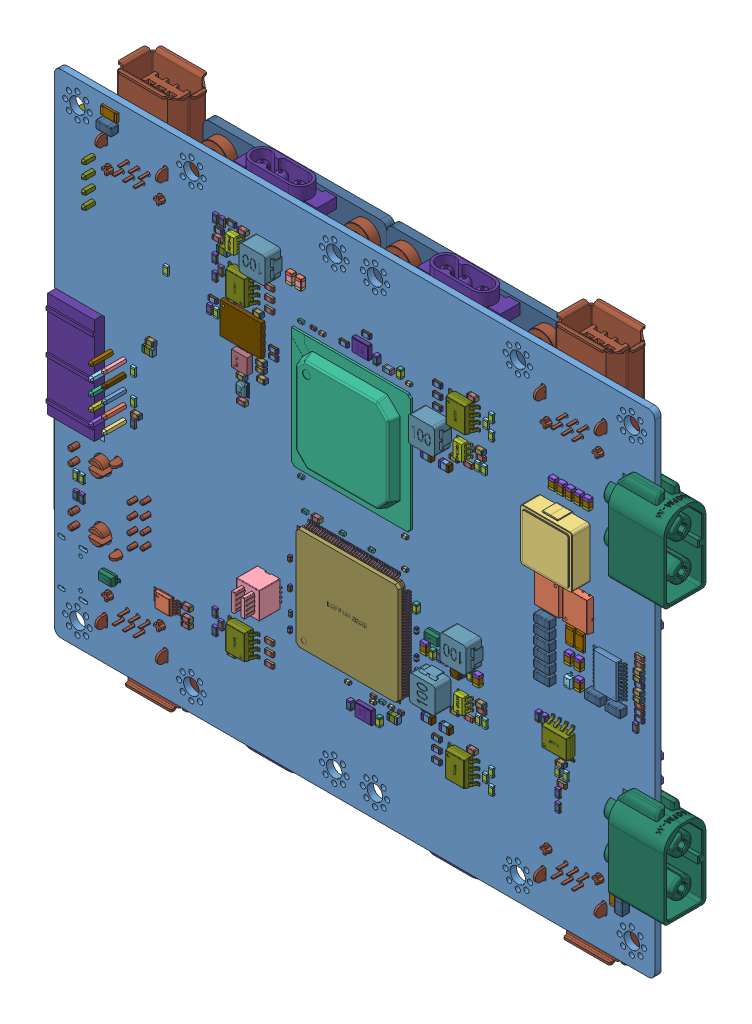
SolidWorks assembly Mother  Board, configuration 默认. Lengths in mm. (continued)
Components (placement in the parent): (continued)
- Mother  Board.step-1: Mother  Board.step [默认] at origin size (122.6 102.08 21) (continued)
  - R4_D2.step-1: R4_D2.step [默认] at origin size (0.8 1.6 0.45) (continued)
    - 5993842864.step-1: 5993842864.step [默认] at (78.9939 13.4621 0) x (0 1 0) z (0 0 1) size (1.6 0.8 0.45) (continued)
      - Terminal-12.step-1: Terminal-12.step [默认] at (-0.8 -0.4 0) size (0.3 0.8 0.45)
        - Open_CASCADE_STEP_translator_6.8_21.2.1-28.step-1: Open_CASCADE_STEP_translator_6.8_21.2.1-28.step [默认] at origin size (0.3 0.8 0.45)
      - Terminal-12.step-2: Terminal-12.step [默认] at (0.8 0.4 0) x (-1 0 0) z (0 0 1) size (0.3 0.8 0.45)
        - Open_CASCADE_STEP_translator_6.8_21.2.1-28.step-1: Open_CASCADE_STEP_translator_6.8_21.2.1-28.step [默认] at origin size (0.3 0.8 0.45)
      - Mid_Body-29.step-1: Mid_Body-29.step [默认] at (-0.8 -0.4 0) size (1.51 0.8 0.36)
      - Mark-30.step-1: Mark-30.step [默认] at (-0.5 -0.4 0.405) size (1 0.8 0.05)
  - R4_D1.step-1: R4_D1.step [默认] at origin size (0.8 1.6 0.45)
    - 5993843024.step-1: 5993843024.step [默认] at (27.9401 13.4619 0) x (0 -1 0) z (0 0 1) size (1.6 0.8 0.45)
      - Terminal-13.step-1: Terminal-13.step [默认] at (-0.8 -0.4 0) size (0.3 0.8 0.45)
        - Open_CASCADE_STEP_translator_6.8_21.2.1-31.step-1: Open_CASCADE_STEP_translator_6.8_21.2.1-31.step [默认] at origin size (0.3 0.8 0.45)
      - Terminal-13.step-2: Terminal-13.step [默认] at (0.8 0.4 0) x (-1 0 0) z (0 0 1) size (0.3 0.8 0.45)
        - Open_CASCADE_STEP_translator_6.8_21.2.1-31.step-1: Open_CASCADE_STEP_translator_6.8_21.2.1-31.step [默认] at origin size (0.3 0.8 0.45)
      - Mid_Body-32.step-1: Mid_Body-32.step [默认] at (-0.8 -0.4 0) size (1.51 0.8 0.36)
      - Mark-33.step-1: Mark-33.step [默认] at (-0.5 -0.4 0.405) size (1 0.8 0.05)
  - R3_D4.step-1: R3_D4.step [默认] at origin size (1.6 0.8 0.45)
    - 5993842144.step-1: 5993842144.step [默认] at (69.7231 72.6441 0) x (1 0 0) z (0 0 1) size (1.6 0.8 0.45)
      - Terminal-10.step-1: Terminal-10.step [默认] at (-0.8 -0.4 0) size (0.3 0.8 0.45)
        - Open_CASCADE_STEP_translator_6.8_21.2.1-22.step-1: Open_CASCADE_STEP_translator_6.8_21.2.1-22.step [默认] at origin size (0.3 0.8 0.45)
      - Terminal-10.step-2: Terminal-10.step [默认] at (0.8 0.4 0) x (-1 0 0) z (0 0 1) size (0.3 0.8 0.45)
        - Open_CASCADE_STEP_translator_6.8_21.2.1-22.step-1: Open_CASCADE_STEP_translator_6.8_21.2.1-22.step [默认] at origin size (0.3 0.8 0.45)
      - Mid_Body-23.step-1: Mid_Body-23.step [默认] at (-0.8 -0.4 0) size (1.51 0.8 0.36)
      - Mark-24.step-1: Mark-24.step [默认] at (-0.5 -0.4 0.405) size (1 0.8 0.05)
  - R3_D3.step-1: R3_D3.step [默认] at origin size (1.6 0.8 0.45)
    - 5993842944.step-1: 5993842944.step [默认] at (37.3379 72.6439 0) x (-1 0 0) z (0 0 1) size (1.6 0.8 0.45)
      - Terminal-14.step-1: Terminal-14.step [默认] at (-0.8 -0.4 0) size (0.3 0.8 0.45)
        - Open_CASCADE_STEP_translator_6.8_21.2.1-34.step-1: Open_CASCADE_STEP_translator_6.8_21.2.1-34.step [默认] at origin size (0.3 0.8 0.45)
      - Terminal-14.step-2: Terminal-14.step [默认] at (0.8 0.4 0) x (-1 0 0) z (0 0 1) size (0.3 0.8 0.45)
        - Open_CASCADE_STEP_translator_6.8_21.2.1-34.step-1: Open_CASCADE_STEP_translator_6.8_21.2.1-34.step [默认] at origin size (0.3 0.8 0.45)
      - Mid_Body-35.step-1: Mid_Body-35.step [默认] at (-0.8 -0.4 0) size (1.51 0.8 0.36)
      - Mark-36.step-1: Mark-36.step [默认] at (-0.5 -0.4 0.405) size (1 0.8 0.05)
  - R3_D2.step-1: R3_D2.step [默认] at origin size (1.6 0.8 0.45)
    - 5993842144.step-1: 5993842144.step [默认] at (69.5961 13.4621 0) x (1 0 0) z (0 0 1) size (1.6 0.8 0.45)
      - Terminal-10.step-1: Terminal-10.step [默认] at (-0.8 -0.4 0) size (0.3 0.8 0.45)
        - Open_CASCADE_STEP_translator_6.8_21.2.1-22.step-1: Open_CASCADE_STEP_translator_6.8_21.2.1-22.step [默认] at origin size (0.3 0.8 0.45)
      - Terminal-10.step-2: Terminal-10.step [默认] at (0.8 0.4 0) x (-1 0 0) z (0 0 1) size (0.3 0.8 0.45)
        - Open_CASCADE_STEP_translator_6.8_21.2.1-22.step-1: Open_CASCADE_STEP_translator_6.8_21.2.1-22.step [默认] at origin size (0.3 0.8 0.45)
      - Mid_Body-23.step-1: Mid_Body-23.step [默认] at (-0.8 -0.4 0) size (1.51 0.8 0.36)
      - Mark-24.step-1: Mark-24.step [默认] at (-0.5 -0.4 0.405) size (1 0.8 0.05)
  - R3_D1.step-1: R3_D1.step [默认] at origin size (1.6 0.8 0.45)
    - 5993842944.step-1: 5993842944.step [默认] at (37.3379 13.4619 0) x (-1 0 0) z (0 0 1) size (1.6 0.8 0.45)
      - Terminal-14.step-1: Terminal-14.step [默认] at (-0.8 -0.4 0) size (0.3 0.8 0.45)
        - Open_CASCADE_STEP_translator_6.8_21.2.1-34.step-1: Open_CASCADE_STEP_translator_6.8_21.2.1-34.step [默认] at origin size (0.3 0.8 0.45)
      - Terminal-14.step-2: Terminal-14.step [默认] at (0.8 0.4 0) x (-1 0 0) z (0 0 1) size (0.3 0.8 0.45)
        - Open_CASCADE_STEP_translator_6.8_21.2.1-34.step-1: Open_CASCADE_STEP_translator_6.8_21.2.1-34.step [默认] at origin size (0.3 0.8 0.45)
      - Mid_Body-35.step-1: Mid_Body-35.step [默认] at (-0.8 -0.4 0) size (1.51 0.8 0.36)
      - Mark-36.step-1: Mark-36.step [默认] at (-0.5 -0.4 0.405) size (1 0.8 0.05)
  - R2_D4.step-1: R2_D4.step [默认] at origin size (1.6 0.8 0.45)
    - 5993842144.step-1: 5993842144.step [默认] at (69.7231 74.5491 0) x (1 0 0) z (0 0 1) size (1.6 0.8 0.45)
      - Terminal-10.step-1: Terminal-10.step [默认] at (-0.8 -0.4 0) size (0.3 0.8 0.45)
        - Open_CASCADE_STEP_translator_6.8_21.2.1-22.step-1: Open_CASCADE_STEP_translator_6.8_21.2.1-22.step [默认] at origin size (0.3 0.8 0.45)
      - Terminal-10.step-2: Terminal-10.step [默认] at (0.8 0.4 0) x (-1 0 0) z (0 0 1) size (0.3 0.8 0.45)
        - Open_CASCADE_STEP_translator_6.8_21.2.1-22.step-1: Open_CASCADE_STEP_translator_6.8_21.2.1-22.step [默认] at origin size (0.3 0.8 0.45)
      - Mid_Body-23.step-1: Mid_Body-23.step [默认] at (-0.8 -0.4 0) size (1.51 0.8 0.36)
      - Mark-24.step-1: Mark-24.step [默认] at (-0.5 -0.4 0.405) size (1 0.8 0.05)
  - R2_D3.step-1: R2_D3.step [默认] at origin size (1.6 0.8 0.45)
    - 5993842944.step-1: 5993842944.step [默认] at (37.3379 70.7389 0) x (-1 0 0) z (0 0 1) size (1.6 0.8 0.45)
      - Terminal-14.step-1: Terminal-14.step [默认] at (-0.8 -0.4 0) size (0.3 0.8 0.45)
        - Open_CASCADE_STEP_translator_6.8_21.2.1-34.step-1: Open_CASCADE_STEP_translator_6.8_21.2.1-34.step [默认] at origin size (0.3 0.8 0.45)
      - Terminal-14.step-2: Terminal-14.step [默认] at (0.8 0.4 0) x (-1 0 0) z (0 0 1) size (0.3 0.8 0.45)
        - Open_CASCADE_STEP_translator_6.8_21.2.1-34.step-1: Open_CASCADE_STEP_translator_6.8_21.2.1-34.step [默认] at origin size (0.3 0.8 0.45)
      - Mid_Body-35.step-1: Mid_Body-35.step [默认] at (-0.8 -0.4 0) size (1.51 0.8 0.36)
      - Mark-36.step-1: Mark-36.step [默认] at (-0.5 -0.4 0.405) size (1 0.8 0.05)
  - R2_D2.step-1: R2_D2.step [默认] at origin size (1.6 0.8 0.45)
    - 5993842144.step-1: 5993842144.step [默认] at (69.5961 15.3671 0) x (1 0 0) z (0 0 1) size (1.6 0.8 0.45)
      - Terminal-10.step-1: Terminal-10.step [默认] at (-0.8 -0.4 0) size (0.3 0.8 0.45)
        - Open_CASCADE_STEP_translator_6.8_21.2.1-22.step-1: Open_CASCADE_STEP_translator_6.8_21.2.1-22.step [默认] at origin size (0.3 0.8 0.45)
      - Terminal-10.step-2: Terminal-10.step [默认] at (0.8 0.4 0) x (-1 0 0) z (0 0 1) size (0.3 0.8 0.45)
        - Open_CASCADE_STEP_translator_6.8_21.2.1-22.step-1: Open_CASCADE_STEP_translator_6.8_21.2.1-22.step [默认] at origin size (0.3 0.8 0.45)
      - Mid_Body-23.step-1: Mid_Body-23.step [默认] at (-0.8 -0.4 0) size (1.51 0.8 0.36)
      - Mark-24.step-1: Mark-24.step [默认] at (-0.5 -0.4 0.405) size (1 0.8 0.05)
  - R2_D1.step-1: R2_D1.step [默认] at origin size (1.6 0.8 0.45)
    - 5993842944.step-1: 5993842944.step [默认] at (37.3379 11.5569 0) x (-1 0 0) z (0 0 1) size (1.6 0.8 0.45)
      - Terminal-14.step-1: Terminal-14.step [默认] at (-0.8 -0.4 0) size (0.3 0.8 0.45)
        - Open_CASCADE_STEP_translator_6.8_21.2.1-34.step-1: Open_CASCADE_STEP_translator_6.8_21.2.1-34.step [默认] at origin size (0.3 0.8 0.45)
      - Terminal-14.step-2: Terminal-14.step [默认] at (0.8 0.4 0) x (-1 0 0) z (0 0 1) size (0.3 0.8 0.45)
        - Open_CASCADE_STEP_translator_6.8_21.2.1-34.step-1: Open_CASCADE_STEP_translator_6.8_21.2.1-34.step [默认] at origin size (0.3 0.8 0.45)
      - Mid_Body-35.step-1: Mid_Body-35.step [默认] at (-0.8 -0.4 0) size (1.51 0.8 0.36)
      - Mark-36.step-1: Mark-36.step [默认] at (-0.5 -0.4 0.405) size (1 0.8 0.05)
  - R1_D4.step-1: R1_D4.step [默认] at origin size (0.8 1.6 0.45)
    - 5993842864.step-1: 5993842864.step [默认] at (80.1369 74.1681 0) x (0 1 0) z (0 0 1) size (1.6 0.8 0.45)
      - Terminal-12.step-1: Terminal-12.step [默认] at (-0.8 -0.4 0) size (0.3 0.8 0.45)
        - Open_CASCADE_STEP_translator_6.8_21.2.1-28.step-1: Open_CASCADE_STEP_translator_6.8_21.2.1-28.step [默认] at origin size (0.3 0.8 0.45)
      - Terminal-12.step-2: Terminal-12.step [默认] at (0.8 0.4 0) x (-1 0 0) z (0 0 1) size (0.3 0.8 0.45)
        - Open_CASCADE_STEP_translator_6.8_21.2.1-28.step-1: Open_CASCADE_STEP_translator_6.8_21.2.1-28.step [默认] at origin size (0.3 0.8 0.45)
      - Mid_Body-29.step-1: Mid_Body-29.step [默认] at (-0.8 -0.4 0) size (1.51 0.8 0.36)
      - Mark-30.step-1: Mark-30.step [默认] at (-0.5 -0.4 0.405) size (1 0.8 0.05)
  - R1_D3.step-1: R1_D3.step [默认] at origin size (0.8 1.6 0.45)
    - 5993843024.step-1: 5993843024.step [默认] at (26.7971 71.1199 0) x (0 -1 0) z (0 0 1) size (1.6 0.8 0.45)
      - Terminal-13.step-1: Terminal-13.step [默认] at (-0.8 -0.4 0) size (0.3 0.8 0.45)
        - Open_CASCADE_STEP_translator_6.8_21.2.1-31.step-1: Open_CASCADE_STEP_translator_6.8_21.2.1-31.step [默认] at origin size (0.3 0.8 0.45)
      - Terminal-13.step-2: Terminal-13.step [默认] at (0.8 0.4 0) x (-1 0 0) z (0 0 1) size (0.3 0.8 0.45)
        - Open_CASCADE_STEP_translator_6.8_21.2.1-31.step-1: Open_CASCADE_STEP_translator_6.8_21.2.1-31.step [默认] at origin size (0.3 0.8 0.45)
      - Mid_Body-32.step-1: Mid_Body-32.step [默认] at (-0.8 -0.4 0) size (1.51 0.8 0.36)
      - Mark-33.step-1: Mark-33.step [默认] at (-0.5 -0.4 0.405) size (1 0.8 0.05)
  - R1_D2.step-1: R1_D2.step [默认] at origin size (0.8 1.6 0.45)
    - 5993842864.step-1: 5993842864.step [默认] at (80.1369 14.9861 0) x (0 1 0) z (0 0 1) size (1.6 0.8 0.45)
      - Terminal-12.step-1: Terminal-12.step [默认] at (-0.8 -0.4 0) size (0.3 0.8 0.45)
        - Open_CASCADE_STEP_translator_6.8_21.2.1-28.step-1: Open_CASCADE_STEP_translator_6.8_21.2.1-28.step [默认] at origin size (0.3 0.8 0.45)
      - Terminal-12.step-2: Terminal-12.step [默认] at (0.8 0.4 0) x (-1 0 0) z (0 0 1) size (0.3 0.8 0.45)
        - Open_CASCADE_STEP_translator_6.8_21.2.1-28.step-1: Open_CASCADE_STEP_translator_6.8_21.2.1-28.step [默认] at origin size (0.3 0.8 0.45)
      - Mid_Body-29.step-1: Mid_Body-29.step [默认] at (-0.8 -0.4 0) size (1.51 0.8 0.36)
      - Mark-30.step-1: Mark-30.step [默认] at (-0.5 -0.4 0.405) size (1 0.8 0.05)
  - R1_D1.step-1: R1_D1.step [默认] at origin size (0.8 1.6 0.45)
    - 5993843024.step-1: 5993843024.step [默认] at (26.7971 11.9379 0) x (0 -1 0) z (0 0 1) size (1.6 0.8 0.45)
      - Terminal-13.step-1: Terminal-13.step [默认] at (-0.8 -0.4 0) size (0.3 0.8 0.45)
        - Open_CASCADE_STEP_translator_6.8_21.2.1-31.step-1: Open_CASCADE_STEP_translator_6.8_21.2.1-31.step [默认] at origin size (0.3 0.8 0.45)
      - Terminal-13.step-2: Terminal-13.step [默认] at (0.8 0.4 0) x (-1 0 0) z (0 0 1) size (0.3 0.8 0.45)
        - Open_CASCADE_STEP_translator_6.8_21.2.1-31.step-1: Open_CASCADE_STEP_translator_6.8_21.2.1-31.step [默认] at origin size (0.3 0.8 0.45)
      - Mid_Body-32.step-1: Mid_Body-32.step [默认] at (-0.8 -0.4 0) size (1.51 0.8 0.36)
      - Mark-33.step-1: Mark-33.step [默认] at (-0.5 -0.4 0.405) size (1 0.8 0.05)
  - M2.step-1: M2.step [默认] at origin size (5.15 6.15 1.1)
    - TDSON-8.step-1: TDSON-8.step [默认] at (97.0281 50.8001 0) x (1 0 0) z (0 -1 0) size (5.15 1.1 6.15)
  - M1.step-1: M1.step [默认] at origin size (5.15 6.15 1.1)
    - TDSON-8.step-1: TDSON-8.step [默认] at (91.5669 50.7999 0) x (-1 0 0) z (0 1 0) size (5.15 1.1 6.15)
  - L5.step-1: L5.step [默认] at origin size (5.6 5 3.1)
    - User_Library-FERROCORE_HPI0530-100.step-1: User_Library-FERROCORE_HPI0530-100.step [默认] at (72.9381 36.2051 0) x (-1 0 0) z (0 1 0) size (5.6 3.1 5)
  - L1.step-1: L1.step [默认] at origin size (10 10.4 3.9)
    - User_Library-SMPI1004HW.step-1: User_Library-SMPI1004HW.step [默认] at (94.2339 61.1089 3.8) x (-1 0 0) z (0 0 -1) size (10 10.4 3.9)
  - JP5.step-1: JP5.step [默认] at origin size (4.96 5.1 6.5)
    - SG340-GxxP-B1-2x4.step-1: SG340-GxxP-B1-2x4.step [默认] at (36.9697 24.1146 0.1) x (0 1 0) z (0 0 1) size (5.1 4.96 6.5)
  - JP1_D4.step-1: JP1_D4.step [默认] at origin size (13.5 16.6 11.9)
    - 1364-6.step-1: 1364-6.step [默认] at (95.766 94.092 -5.9164) x (1 0 0) z (0 1 0) size (13.5 11.9 16.6)
  - JP2_D4.step-1: JP2_D4.step [默认] at origin size (11.5 5 4.6)
    - SG340-GxxS-B1-2x12.step-1: SG340-GxxS-B1-2x12.step [默认] at (71.1836 47.117 -1.3164) x (-1 0 0) z (0 0 -1) size (11.5 5 4.6)
  - FB1.step-1: FB1.step [默认] at origin size (0.8 1.6 0.8)
    - 742792606.step-1: 742792606.step [默认] at (16.5101 12.9541 -1.6064) x (1 0 0) z (0 0 -1) size (0.8 0.3 0.8)
    - 742792606-48.step-1: 742792606-48.step [默认] at (16.5101 12.9541 -1.6064) x (1 0 0) z (0 0 -1) size (0.8 0.3 0.8)
    - 742792606-49.step-1: 742792606-49.step [默认] at (16.5101 12.9541 -1.6064) x (1 0 0) z (0 0 -1) size (0.8 1 0.8)
  - D2.step-1: D2.step [默认] at origin size (3.7 1.6 1.22)
    - SOD-123.step-1: SOD-123.step [默认] at (69.342 32.258 0.05) x (1 0 0) z (0 0 1) size (3.7 1.6 1.22)
      - SOD-123-50.step-1: SOD-123-50.step [默认] at origin size (3.7 1.6 1.22)
      - LOGO______.__.step-1: LOGO______.__.step [默认] at (-0.0155 0.0364 -0.003) x (-1 0 0) z (0 0 -1) size (0.9 1.04 0.01)
  - D1.step-1: D1.step [默认] at origin size (1.3 2.65 0.96)
    - SOD-323.step-1: SOD-323.step [默认] at (95.396 37.8588 0.05) x (0 1 0) z (0 0 1) size (2.65 1.3 0.96)
      - SOD-323-71.step-1: SOD-323-71.step [默认] at origin size (2.65 1.3 0.95)
      - LOGO______.__-72.step-1: LOGO______.__-72.step [默认] at (0.0033 0.0815 -0.003) x (-1 0 0) z (0 0 -1) size (0.9 1.04 0.01)
  - CP8.step-1: CP8.step [默认] at origin size (3 1.5 1.5)
    - (______).step-1: (______).step [默认] at (90.9377 36.556 0) x (0 1 0) z (0 0 1) size (1.5 3 1.5)
  - CP7.step-1: CP7.step [默认] at origin size (3 1.5 1.5)
    - (______).step-1: (______).step [默认] at (90.9377 44.176 0) x (0 1 0) z (0 0 1) size (1.5 3 1.5)
  - CP6.step-1: CP6.step [默认] at origin size (3 1.5 1.5)
    - (______).step-1: (______).step [默认] at (90.9377 42.271 0) x (0 1 0) z (0 0 1) size (1.5 3 1.5)
  - CP5.step-1: CP5.step [默认] at origin size (3 1.5 1.5)
    - (______).step-1: (______).step [默认] at (90.9377 40.366 0) x (0 1 0) z (0 0 1) size (1.5 3 1.5)
  - CP4.step-1: CP4.step [默认] at origin size (3 1.5 1.5)
    - (______).step-1: (______).step [默认] at (90.9377 38.461 0) x (0 1 0) z (0 0 1) size (1.5 3 1.5)
  - CP3.step-1: CP3.step [默认] at origin size (3 1.5 1.5)
    - (______).step-1: (______).step [默认] at (90.9375 46.0808 0) x (0 -1 0) z (0 0 1) size (1.5 3 1.5)
  - CP2.step-1: CP2.step [默认] at origin size (3 1.5 1.5)
    - (______).step-1: (______).step [默认] at (104.6479 38.0999 0) x (0 -1 0) z (0 0 1) size (1.5 3 1.5)
  - CP1.step-1: CP1.step [默认] at origin size (3 1.5 1.5)
    - (______).step-1: (______).step [默认] at (100.7109 38.0999 0) x (0 -1 0) z (0 0 1) size (1.5 3 1.5)
  - C56.step-1: C56.step [默认] at origin size (1.6 0.8 0.8)
    - 5993854224.step-1: 5993854224.step [默认] at (21.5901 10.4141 0) x (1 0 0) z (0 0 1) size (1.6 0.8 0.8)
      - Terminal-17.step-1: Terminal-17.step [默认] at (-0.8 -0.4 0) size (1.6 0.8 0.8)
        - Open_CASCADE_STEP_translator_6.8_47.1.1-60.step-1: Open_CASCADE_STEP_translator_6.8_47.1.1-60.step [默认] at origin size (0.3 0.8 0.8)
        - Open_CASCADE_STEP_translator_6.8_47.1.2-61.step-1: Open_CASCADE_STEP_translator_6.8_47.1.2-61.step [默认] at origin size (0.3 0.8 0.8)
      - Mid_Body-8.step-1: Mid_Body-8.step [默认] at (-0.8 -0.4 0) size (1 0.8 0.8)
        - Open_CASCADE_STEP_translator_6.8_47.2.1-62.step-1: Open_CASCADE_STEP_translator_6.8_47.2.1-62.step [默认] at origin size (1 0.8 0.8)
  - C55.step-1: C55.step [默认] at origin size (1.6 0.8 0.8)
    - 5993854224.step-1: 5993854224.step [默认] at (21.5901 11.4301 0) x (1 0 0) z (0 0 1) size (1.6 0.8 0.8)
      - Terminal-17.step-1: Terminal-17.step [默认] at (-0.8 -0.4 0) size (1.6 0.8 0.8)
        - Open_CASCADE_STEP_translator_6.8_47.1.1-60.step-1: Open_CASCADE_STEP_translator_6.8_47.1.1-60.step [默认] at origin size (0.3 0.8 0.8)
        - Open_CASCADE_STEP_translator_6.8_47.1.2-61.step-1: Open_CASCADE_STEP_translator_6.8_47.1.2-61.step [默认] at origin size (0.3 0.8 0.8)
      - Mid_Body-8.step-1: Mid_Body-8.step [默认] at (-0.8 -0.4 0) size (1 0.8 0.8)
        - Open_CASCADE_STEP_translator_6.8_47.2.1-62.step-1: Open_CASCADE_STEP_translator_6.8_47.2.1-62.step [默认] at origin size (1 0.8 0.8)
  - C54.step-1: C54.step [默认] at origin size (1.6 0.8 0.8)
    - 5993854224.step-1: 5993854224.step [默认] at (21.5901 13.3351 0) x (1 0 0) z (0 0 1) size (1.6 0.8 0.8)
      - Terminal-17.step-1: Terminal-17.step [默认] at (-0.8 -0.4 0) size (1.6 0.8 0.8)
        - Open_CASCADE_STEP_translator_6.8_47.1.1-60.step-1: Open_CASCADE_STEP_translator_6.8_47.1.1-60.step [默认] at origin size (0.3 0.8 0.8)
        - Open_CASCADE_STEP_translator_6.8_47.1.2-61.step-1: Open_CASCADE_STEP_translator_6.8_47.1.2-61.step [默认] at origin size (0.3 0.8 0.8)
      - Mid_Body-8.step-1: Mid_Body-8.step [默认] at (-0.8 -0.4 0) size (1 0.8 0.8)
        - Open_CASCADE_STEP_translator_6.8_47.2.1-62.step-1: Open_CASCADE_STEP_translator_6.8_47.2.1-62.step [默认] at origin size (1 0.8 0.8)
  - C53.step-1: C53.step [默认] at origin size (0.8 1.6 0.8)
    - 5993843264.step-1: 5993843264.step [默认] at (20.7009 25.5317 -1.2164) x (0 1 0) z (0 0 -1) size (1.6 0.8 0.8)
      - Terminal-16.step-1: Terminal-16.step [默认] at (-0.8 -0.4 0) size (1.6 0.8 0.8)
        - Open_CASCADE_STEP_translator_6.8_47.1.1-57.step-1: Open_CASCADE_STEP_translator_6.8_47.1.1-57.step [默认] at origin size (0.3 0.8 0.8)
        - Open_CASCADE_STEP_translator_6.8_47.1.2-58.step-1: Open_CASCADE_STEP_translator_6.8_47.1.2-58.step [默认] at origin size (0.3 0.8 0.8)
      - Mid_Body-7.step-1: Mid_Body-7.step [默认] at (-0.8 -0.4 0) size (1 0.8 0.8)
        - Open_CASCADE_STEP_translator_6.8_47.2.1-59.step-1: Open_CASCADE_STEP_translator_6.8_47.2.1-59.step [默认] at origin size (1 0.8 0.8)
  - C52.step-1: C52.step [默认] at origin size (0.8 1.6 0.8)
    - 5993853744.step-1: 5993853744.step [默认] at (19.5578 17.1449 -1.2164) x (0 -1 0) z (0 0 -1) size (1.6 0.8 0.8)
      - Terminal-15.step-1: Terminal-15.step [默认] at (-0.8 -0.4 0) size (1.6 0.8 0.8)
        - Open_CASCADE_STEP_translator_6.8_47.1.1-54.step-1: Open_CASCADE_STEP_translator_6.8_47.1.1-54.step [默认] at origin size (0.3 0.8 0.8)
        - Open_CASCADE_STEP_translator_6.8_47.1.2-55.step-1: Open_CASCADE_STEP_translator_6.8_47.1.2-55.step [默认] at origin size (0.3 0.8 0.8)
      - Mid_Body-6.step-1: Mid_Body-6.step [默认] at (-0.8 -0.4 0) size (1 0.8 0.8)
        - Open_CASCADE_STEP_translator_6.8_47.2.1-56.step-1: Open_CASCADE_STEP_translator_6.8_47.2.1-56.step [默认] at origin size (1 0.8 0.8)
  - C51.step-1: C51.step [默认] at origin size (0.8 1.6 0.8)
    - 5993843264.step-1: 5993843264.step [默认] at (25.3999 25.5317 -1.2164) x (0 1 0) z (0 0 -1) size (1.6 0.8 0.8)
      - Terminal-16.step-1: Terminal-16.step [默认] at (-0.8 -0.4 0) size (1.6 0.8 0.8)
        - Open_CASCADE_STEP_translator_6.8_47.1.1-57.step-1: Open_CASCADE_STEP_translator_6.8_47.1.1-57.step [默认] at origin size (0.3 0.8 0.8)
        - Open_CASCADE_STEP_translator_6.8_47.1.2-58.step-1: Open_CASCADE_STEP_translator_6.8_47.1.2-58.step [默认] at origin size (0.3 0.8 0.8)
      - Mid_Body-7.step-1: Mid_Body-7.step [默认] at (-0.8 -0.4 0) size (1 0.8 0.8)
        - Open_CASCADE_STEP_translator_6.8_47.2.1-59.step-1: Open_CASCADE_STEP_translator_6.8_47.2.1-59.step [默认] at origin size (1 0.8 0.8)
  - C50.step-1: C50.step [默认] at origin size (0.8 1.6 0.8)
    - 5993843264.step-1: 5993843264.step [默认] at (24.2569 25.5317 -1.2164) x (0 1 0) z (0 0 -1) size (1.6 0.8 0.8)
      - Terminal-16.step-1: Terminal-16.step [默认] at (-0.8 -0.4 0) size (1.6 0.8 0.8)
        - Open_CASCADE_STEP_translator_6.8_47.1.1-57.step-1: Open_CASCADE_STEP_translator_6.8_47.1.1-57.step [默认] at origin size (0.3 0.8 0.8)
        - Open_CASCADE_STEP_translator_6.8_47.1.2-58.step-1: Open_CASCADE_STEP_translator_6.8_47.1.2-58.step [默认] at origin size (0.3 0.8 0.8)
      - Mid_Body-7.step-1: Mid_Body-7.step [默认] at (-0.8 -0.4 0) size (1 0.8 0.8)
        - Open_CASCADE_STEP_translator_6.8_47.2.1-59.step-1: Open_CASCADE_STEP_translator_6.8_47.2.1-59.step [默认] at origin size (1 0.8 0.8)
  - C49.step-1: C49.step [默认] at origin size (0.8 1.6 0.8)
    - 5993843264.step-1: 5993843264.step [默认] at (25.1461 28.8291 -1.2164) x (0 1 0) z (0 0 -1) size (1.6 0.8 0.8)
      - Terminal-16.step-1: Terminal-16.step [默认] at (-0.8 -0.4 0) size (1.6 0.8 0.8)
        - Open_CASCADE_STEP_translator_6.8_47.1.1-57.step-1: Open_CASCADE_STEP_translator_6.8_47.1.1-57.step [默认] at origin size (0.3 0.8 0.8)
        - Open_CASCADE_STEP_translator_6.8_47.1.2-58.step-1: Open_CASCADE_STEP_translator_6.8_47.1.2-58.step [默认] at origin size (0.3 0.8 0.8)
      - Mid_Body-7.step-1: Mid_Body-7.step [默认] at (-0.8 -0.4 0) size (1 0.8 0.8)
        - Open_CASCADE_STEP_translator_6.8_47.2.1-59.step-1: Open_CASCADE_STEP_translator_6.8_47.2.1-59.step [默认] at origin size (1 0.8 0.8)
  - C48.step-1: C48.step [默认] at origin size (0.8 1.6 0.8)
    - 5993853744.step-1: 5993853744.step [默认] at (19.5579 28.8289 -1.2164) x (0 -1 0) z (0 0 -1) size (1.6 0.8 0.8)
      - Terminal-15.step-1: Terminal-15.step [默认] at (-0.8 -0.4 0) size (1.6 0.8 0.8)
        - Open_CASCADE_STEP_translator_6.8_47.1.1-54.step-1: Open_CASCADE_STEP_translator_6.8_47.1.1-54.step [默认] at origin size (0.3 0.8 0.8)
        - Open_CASCADE_STEP_translator_6.8_47.1.2-55.step-1: Open_CASCADE_STEP_translator_6.8_47.1.2-55.step [默认] at origin size (0.3 0.8 0.8)
      - Mid_Body-6.step-1: Mid_Body-6.step [默认] at (-0.8 -0.4 0) size (1 0.8 0.8)
        - Open_CASCADE_STEP_translator_6.8_47.2.1-56.step-1: Open_CASCADE_STEP_translator_6.8_47.2.1-56.step [默认] at origin size (1 0.8 0.8)
  - C47.step-1: C47.step [默认] at origin size (1.6 0.8 0.8)
    - 5993853264.step-1: 5993853264.step [默认] at (17.2719 15.2401 -1.2164) x (-1 0 0) z (0 0 -1) size (1.6 0.8 0.8)
      - Terminal-6.step-1: Terminal-6.step [默认] at (-0.8 -0.4 0) size (1.6 0.8 0.8)
        - Open_CASCADE_STEP_translator_6.8_47.1.1-10.step-1: Open_CASCADE_STEP_translator_6.8_47.1.1-10.step [默认] at origin size (0.3 0.8 0.8)
        - Open_CASCADE_STEP_translator_6.8_47.1.2-11.step-1: Open_CASCADE_STEP_translator_6.8_47.1.2-11.step [默认] at origin size (0.3 0.8 0.8)
      - Mid_Body-5.step-1: Mid_Body-5.step [默认] at (-0.8 -0.4 0) size (1 0.8 0.8)
        - Open_CASCADE_STEP_translator_6.8_47.2.1-12.step-1: Open_CASCADE_STEP_translator_6.8_47.2.1-12.step [默认] at origin size (1 0.8 0.8)
  - C46.step-1: C46.step [默认] at origin size (1.6 0.8 0.8)
    - 5993853264.step-1: 5993853264.step [默认] at (18.7959 12.0651 -1.2164) x (-1 0 0) z (0 0 -1) size (1.6 0.8 0.8)
      - Terminal-6.step-1: Terminal-6.step [默认] at (-0.8 -0.4 0) size (1.6 0.8 0.8)
        - Open_CASCADE_STEP_translator_6.8_47.1.1-10.step-1: Open_CASCADE_STEP_translator_6.8_47.1.1-10.step [默认] at origin size (0.3 0.8 0.8)
        - Open_CASCADE_STEP_translator_6.8_47.1.2-11.step-1: Open_CASCADE_STEP_translator_6.8_47.1.2-11.step [默认] at origin size (0.3 0.8 0.8)
      - Mid_Body-5.step-1: Mid_Body-5.step [默认] at (-0.8 -0.4 0) size (1 0.8 0.8)
        - Open_CASCADE_STEP_translator_6.8_47.2.1-12.step-1: Open_CASCADE_STEP_translator_6.8_47.2.1-12.step [默认] at origin size (1 0.8 0.8)
  - C45.step-1: C45.step [默认] at origin size (1.6 0.8 0.8)
    - 5993853264.step-1: 5993853264.step [默认] at (17.2718 21.3407 -1.2164) x (-1 0 0) z (0 0 -1) size (1.6 0.8 0.8)
      - Terminal-6.step-1: Terminal-6.step [默认] at (-0.8 -0.4 0) size (1.6 0.8 0.8)
        - Open_CASCADE_STEP_translator_6.8_47.1.1-10.step-1: Open_CASCADE_STEP_translator_6.8_47.1.1-10.step [默认] at origin size (0.3 0.8 0.8)
        - Open_CASCADE_STEP_translator_6.8_47.1.2-11.step-1: Open_CASCADE_STEP_translator_6.8_47.1.2-11.step [默认] at origin size (0.3 0.8 0.8)
      - Mid_Body-5.step-1: Mid_Body-5.step [默认] at (-0.8 -0.4 0) size (1 0.8 0.8)
        - Open_CASCADE_STEP_translator_6.8_47.2.1-12.step-1: Open_CASCADE_STEP_translator_6.8_47.2.1-12.step [默认] at origin size (1 0.8 0.8)
  - C44.step-1: C44.step [默认] at origin size (0.8 1.6 0.8)
    - 5993843264.step-1: 5993843264.step [默认] at (18.0339 23.1187 -1.2164) x (0 1 0) z (0 0 -1) size (1.6 0.8 0.8)
      - Terminal-16.step-1: Terminal-16.step [默认] at (-0.8 -0.4 0) size (1.6 0.8 0.8)
        - Open_CASCADE_STEP_translator_6.8_47.1.1-57.step-1: Open_CASCADE_STEP_translator_6.8_47.1.1-57.step [默认] at origin size (0.3 0.8 0.8)
        - Open_CASCADE_STEP_translator_6.8_47.1.2-58.step-1: Open_CASCADE_STEP_translator_6.8_47.1.2-58.step [默认] at origin size (0.3 0.8 0.8)
      - Mid_Body-7.step-1: Mid_Body-7.step [默认] at (-0.8 -0.4 0) size (1 0.8 0.8)
        - Open_CASCADE_STEP_translator_6.8_47.2.1-59.step-1: Open_CASCADE_STEP_translator_6.8_47.2.1-59.step [默认] at origin size (1 0.8 0.8)
  - C43.step-1: C43.step [默认] at origin size (0.8 1.6 0.8)
    - 5993853744.step-1: 5993853744.step [默认] at (18.0338 25.5315 -1.2164) x (0 -1 0) z (0 0 -1) size (1.6 0.8 0.8)
      - Terminal-15.step-1: Terminal-15.step [默认] at (-0.8 -0.4 0) size (1.6 0.8 0.8)
        - Open_CASCADE_STEP_translator_6.8_47.1.1-54.step-1: Open_CASCADE_STEP_translator_6.8_47.1.1-54.step [默认] at origin size (0.3 0.8 0.8)
        - Open_CASCADE_STEP_translator_6.8_47.1.2-55.step-1: Open_CASCADE_STEP_translator_6.8_47.1.2-55.step [默认] at origin size (0.3 0.8 0.8)
      - Mid_Body-6.step-1: Mid_Body-6.step [默认] at (-0.8 -0.4 0) size (1 0.8 0.8)
        - Open_CASCADE_STEP_translator_6.8_47.2.1-56.step-1: Open_CASCADE_STEP_translator_6.8_47.2.1-56.step [默认] at origin size (1 0.8 0.8)
  - C42.step-1: C42.step [默认] at origin size (0.8 1.6 0.8)
    - 5993843264.step-1: 5993843264.step [默认] at (18.0339 17.1497 -1.2164) x (0 1 0) z (0 0 -1) size (1.6 0.8 0.8)
      - Terminal-16.step-1: Terminal-16.step [默认] at (-0.8 -0.4 0) size (1.6 0.8 0.8)
        - Open_CASCADE_STEP_translator_6.8_47.1.1-57.step-1: Open_CASCADE_STEP_translator_6.8_47.1.1-57.step [默认] at origin size (0.3 0.8 0.8)
        - Open_CASCADE_STEP_translator_6.8_47.1.2-58.step-1: Open_CASCADE_STEP_translator_6.8_47.1.2-58.step [默认] at origin size (0.3 0.8 0.8)
      - Mid_Body-7.step-1: Mid_Body-7.step [默认] at (-0.8 -0.4 0) size (1 0.8 0.8)
        - Open_CASCADE_STEP_translator_6.8_47.2.1-59.step-1: Open_CASCADE_STEP_translator_6.8_47.2.1-59.step [默认] at origin size (1 0.8 0.8)
  - C41.step-1: C41.step [默认] at origin size (0.8 1.6 0.8)
    - 5993853744.step-1: 5993853744.step [默认] at (18.0338 19.5626 -1.2164) x (0 -1 0) z (0 0 -1) size (1.6 0.8 0.8)
      - Terminal-15.step-1: Terminal-15.step [默认] at (-0.8 -0.4 0) size (1.6 0.8 0.8)
        - Open_CASCADE_STEP_translator_6.8_47.1.1-54.step-1: Open_CASCADE_STEP_translator_6.8_47.1.1-54.step [默认] at origin size (0.3 0.8 0.8)
        - Open_CASCADE_STEP_translator_6.8_47.1.2-55.step-1: Open_CASCADE_STEP_translator_6.8_47.1.2-55.step [默认] at origin size (0.3 0.8 0.8)
      - Mid_Body-6.step-1: Mid_Body-6.step [默认] at (-0.8 -0.4 0) size (1 0.8 0.8)
        - Open_CASCADE_STEP_translator_6.8_47.2.1-56.step-1: Open_CASCADE_STEP_translator_6.8_47.2.1-56.step [默认] at origin size (1 0.8 0.8)
  - C40.step-1: C40.step [默认] at origin size (1.6 0.8 0.8)
    - 5993853264.step-1: 5993853264.step [默认] at (35.9409 60.1979 0) x (-1 0 0) z (0 0 1) size (1.6 0.8 0.8)
      - Terminal-6.step-1: Terminal-6.step [默认] at (-0.8 -0.4 0) size (1.6 0.8 0.8)
        - Open_CASCADE_STEP_translator_6.8_47.1.1-10.step-1: Open_CASCADE_STEP_translator_6.8_47.1.1-10.step [默认] at origin size (0.3 0.8 0.8)
        - Open_CASCADE_STEP_translator_6.8_47.1.2-11.step-1: Open_CASCADE_STEP_translator_6.8_47.1.2-11.step [默认] at origin size (0.3 0.8 0.8)
      - Mid_Body-5.step-1: Mid_Body-5.step [默认] at (-0.8 -0.4 0) size (1 0.8 0.8)
        - Open_CASCADE_STEP_translator_6.8_47.2.1-12.step-1: Open_CASCADE_STEP_translator_6.8_47.2.1-12.step [默认] at origin size (1 0.8 0.8)
  - C39.step-1: C39.step [默认] at origin size (1.6 0.8 0.8)
    - 5993853264.step-1: 5993853264.step [默认] at (36.0679 58.5469 0) x (-1 0 0) z (0 0 1) size (1.6 0.8 0.8)
      - Terminal-6.step-1: Terminal-6.step [默认] at (-0.8 -0.4 0) size (1.6 0.8 0.8)
        - Open_CASCADE_STEP_translator_6.8_47.1.1-10.step-1: Open_CASCADE_STEP_translator_6.8_47.1.1-10.step [默认] at origin size (0.3 0.8 0.8)
        - Open_CASCADE_STEP_translator_6.8_47.1.2-11.step-1: Open_CASCADE_STEP_translator_6.8_47.1.2-11.step [默认] at origin size (0.3 0.8 0.8)
      - Mid_Body-5.step-1: Mid_Body-5.step [默认] at (-0.8 -0.4 0) size (1 0.8 0.8)
        - Open_CASCADE_STEP_translator_6.8_47.2.1-12.step-1: Open_CASCADE_STEP_translator_6.8_47.2.1-12.step [默认] at origin size (1 0.8 0.8)
  - C38.step-1: C38.step [默认] at origin size (1.6 0.8 0.8)
    - 5993853264.step-1: 5993853264.step [默认] at (35.9409 61.3409 0) x (-1 0 0) z (0 0 1) size (1.6 0.8 0.8)
      - Terminal-6.step-1: Terminal-6.step [默认] at (-0.8 -0.4 0) size (1.6 0.8 0.8)
        - Open_CASCADE_STEP_translator_6.8_47.1.1-10.step-1: Open_CASCADE_STEP_translator_6.8_47.1.1-10.step [默认] at origin size (0.3 0.8 0.8)
        - Open_CASCADE_STEP_translator_6.8_47.1.2-11.step-1: Open_CASCADE_STEP_translator_6.8_47.1.2-11.step [默认] at origin size (0.3 0.8 0.8)
      - Mid_Body-5.step-1: Mid_Body-5.step [默认] at (-0.8 -0.4 0) size (1 0.8 0.8)
        - Open_CASCADE_STEP_translator_6.8_47.2.1-12.step-1: Open_CASCADE_STEP_translator_6.8_47.2.1-12.step [默认] at origin size (1 0.8 0.8)
  - C37.step-1: C37.step [默认] at origin size (1.6 0.8 0.8)
    - 5993854224.step-1: 5993854224.step [默认] at (32.2581 52.9591 0) x (1 0 0) z (0 0 1) size (1.6 0.8 0.8)
      - Terminal-17.step-1: Terminal-17.step [默认] at (-0.8 -0.4 0) size (1.6 0.8 0.8)
        - Open_CASCADE_STEP_translator_6.8_47.1.1-60.step-1: Open_CASCADE_STEP_translator_6.8_47.1.1-60.step [默认] at origin size (0.3 0.8 0.8)
        - Open_CASCADE_STEP_translator_6.8_47.1.2-61.step-1: Open_CASCADE_STEP_translator_6.8_47.1.2-61.step [默认] at origin size (0.3 0.8 0.8)
      - Mid_Body-8.step-1: Mid_Body-8.step [默认] at (-0.8 -0.4 0) size (1 0.8 0.8)
        - Open_CASCADE_STEP_translator_6.8_47.2.1-62.step-1: Open_CASCADE_STEP_translator_6.8_47.2.1-62.step [默认] at origin size (1 0.8 0.8)
  - C36.step-1: C36.step [默认] at origin size (1.6 0.8 0.8)
    - 5993853264.step-1: 5993853264.step [默认] at (32.1309 57.1499 0) x (-1 0 0) z (0 0 1) size (1.6 0.8 0.8)
      - Terminal-6.step-1: Terminal-6.step [默认] at (-0.8 -0.4 0) size (1.6 0.8 0.8)
        - Open_CASCADE_STEP_translator_6.8_47.1.1-10.step-1: Open_CASCADE_STEP_translator_6.8_47.1.1-10.step [默认] at origin size (0.3 0.8 0.8)
        - Open_CASCADE_STEP_translator_6.8_47.1.2-11.step-1: Open_CASCADE_STEP_translator_6.8_47.1.2-11.step [默认] at origin size (0.3 0.8 0.8)
      - Mid_Body-5.step-1: Mid_Body-5.step [默认] at (-0.8 -0.4 0) size (1 0.8 0.8)
        - Open_CASCADE_STEP_translator_6.8_47.2.1-12.step-1: Open_CASCADE_STEP_translator_6.8_47.2.1-12.step [默认] at origin size (1 0.8 0.8)
  - C35.step-1: C35.step [默认] at origin size (0.8 1.6 0.8)
    - 5993843264.step-1: 5993843264.step [默认] at (90.5511 29.0829 0) x (0 -1 0) z (0 0 1) size (1.6 0.8 0.8)
      - Terminal-16.step-1: Terminal-16.step [默认] at (-0.8 -0.4 0) size (1.6 0.8 0.8)
        - Open_CASCADE_STEP_translator_6.8_47.1.1-57.step-1: Open_CASCADE_STEP_translator_6.8_47.1.1-57.step [默认] at origin size (0.3 0.8 0.8)
        - Open_CASCADE_STEP_translator_6.8_47.1.2-58.step-1: Open_CASCADE_STEP_translator_6.8_47.1.2-58.step [默认] at origin size (0.3 0.8 0.8)
      - Mid_Body-7.step-1: Mid_Body-7.step [默认] at (-0.8 -0.4 0) size (1 0.8 0.8)
        - Open_CASCADE_STEP_translator_6.8_47.2.1-59.step-1: Open_CASCADE_STEP_translator_6.8_47.2.1-59.step [默认] at origin size (1 0.8 0.8)
  - C34.step-1: C34.step [默认] at origin size (0.8 1.6 0.8)
    - 5993843264.step-1: 5993843264.step [默认] at (89.4081 29.0829 0) x (0 -1 0) z (0 0 1) size (1.6 0.8 0.8)
      - Terminal-16.step-1: Terminal-16.step [默认] at (-0.8 -0.4 0) size (1.6 0.8 0.8)
        - Open_CASCADE_STEP_translator_6.8_47.1.1-57.step-1: Open_CASCADE_STEP_translator_6.8_47.1.1-57.step [默认] at origin size (0.3 0.8 0.8)
        - Open_CASCADE_STEP_translator_6.8_47.1.2-58.step-1: Open_CASCADE_STEP_translator_6.8_47.1.2-58.step [默认] at origin size (0.3 0.8 0.8)
      - Mid_Body-7.step-1: Mid_Body-7.step [默认] at (-0.8 -0.4 0) size (1 0.8 0.8)
        - Open_CASCADE_STEP_translator_6.8_47.2.1-59.step-1: Open_CASCADE_STEP_translator_6.8_47.2.1-59.step [默认] at origin size (1 0.8 0.8)
  - C33.step-1: C33.step [默认] at origin size (1.6 0.8 0.8)
    - 5993853264.step-1: 5993853264.step [默认] at (93.7259 23.2409 0) x (-1 0 0) z (0 0 1) size (1.6 0.8 0.8)
      - Terminal-6.step-1: Terminal-6.step [默认] at (-0.8 -0.4 0) size (1.6 0.8 0.8)
        - Open_CASCADE_STEP_translator_6.8_47.1.1-10.step-1: Open_CASCADE_STEP_translator_6.8_47.1.1-10.step [默认] at origin size (0.3 0.8 0.8)
        - Open_CASCADE_STEP_translator_6.8_47.1.2-11.step-1: Open_CASCADE_STEP_translator_6.8_47.1.2-11.step [默认] at origin size (0.3 0.8 0.8)
      - Mid_Body-5.step-1: Mid_Body-5.step [默认] at (-0.8 -0.4 0) size (1 0.8 0.8)
        - Open_CASCADE_STEP_translator_6.8_47.2.1-12.step-1: Open_CASCADE_STEP_translator_6.8_47.2.1-12.step [默认] at origin size (1 0.8 0.8)
  - C32.step-1: C32.step [默认] at origin size (0.8 1.6 0.8)
    - 5993853744.step-1: 5993853744.step [默认] at (76.3269 29.3371 0) x (0 1 0) z (0 0 1) size (1.6 0.8 0.8)
      - Terminal-15.step-1: Terminal-15.step [默认] at (-0.8 -0.4 0) size (1.6 0.8 0.8)
        - Open_CASCADE_STEP_translator_6.8_47.1.1-54.step-1: Open_CASCADE_STEP_translator_6.8_47.1.1-54.step [默认] at origin size (0.3 0.8 0.8)
        - Open_CASCADE_STEP_translator_6.8_47.1.2-55.step-1: Open_CASCADE_STEP_translator_6.8_47.1.2-55.step [默认] at origin size (0.3 0.8 0.8)
      - Mid_Body-6.step-1: Mid_Body-6.step [默认] at (-0.8 -0.4 0) size (1 0.8 0.8)
        - Open_CASCADE_STEP_translator_6.8_47.2.1-56.step-1: Open_CASCADE_STEP_translator_6.8_47.2.1-56.step [默认] at origin size (1 0.8 0.8)
  - C31.step-1: C31.step [默认] at origin size (1.25 2.01 0.94)
    - 5993853504.step-1: 5993853504.step [默认] at (77.7239 29.3371 0) x (0 1 0) z (0 0 1) size (2.01 1.25 0.94)
      - Fillet1-73.step-1: Fillet1-73.step [默认] at origin size (0.5 1.25 0.94)
      - Fillet2-74.step-1: Fillet2-74.step [默认] at origin size (0.5 1.25 0.94)
      - body2-75.step-1: body2-75.step [默认] at origin size (1.01 1.22 0.92)
  - C30.step-1: C30.step [默认] at origin size (1.25 2.01 0.94)
    - 5993853504.step-1: 5993853504.step [默认] at (67.5639 29.5911 0) x (0 1 0) z (0 0 1) size (2.01 1.25 0.94)
      - Fillet1-73.step-1: Fillet1-73.step [默认] at origin size (0.5 1.25 0.94)
      - Fillet2-74.step-1: Fillet2-74.step [默认] at origin size (0.5 1.25 0.94)
      - body2-75.step-1: body2-75.step [默认] at origin size (1.01 1.22 0.92)
  - C29.step-1: C29.step [默认] at origin size (0.8 1.6 0.8)
    - 5993853744.step-1: 5993853744.step [默认] at (68.9609 29.2101 0) x (0 1 0) z (0 0 1) size (1.6 0.8 0.8)
      - Terminal-15.step-1: Terminal-15.step [默认] at (-0.8 -0.4 0) size (1.6 0.8 0.8)
        - Open_CASCADE_STEP_translator_6.8_47.1.1-54.step-1: Open_CASCADE_STEP_translator_6.8_47.1.1-54.step [默认] at origin size (0.3 0.8 0.8)
        - Open_CASCADE_STEP_translator_6.8_47.1.2-55.step-1: Open_CASCADE_STEP_translator_6.8_47.1.2-55.step [默认] at origin size (0.3 0.8 0.8)
      - Mid_Body-6.step-1: Mid_Body-6.step [默认] at (-0.8 -0.4 0) size (1 0.8 0.8)
        - Open_CASCADE_STEP_translator_6.8_47.2.1-56.step-1: Open_CASCADE_STEP_translator_6.8_47.2.1-56.step [默认] at origin size (1 0.8 0.8)
  - C13.step-1: C13.step [默认] at origin size (1.25 2.01 0.94)
    - 5993853504.step-1: 5993853504.step [默认] at (95.3769 41.7831 0) x (0 1 0) z (0 0 1) size (2.01 1.25 0.94)
      - Fillet1-73.step-1: Fillet1-73.step [默认] at origin size (0.5 1.25 0.94)
      - Fillet2-74.step-1: Fillet2-74.step [默认] at origin size (0.5 1.25 0.94)
      - body2-75.step-1: body2-75.step [默认] at origin size (1.01 1.22 0.92)
  - C12.step-1: C12.step [默认] at origin size (1.25 2.01 0.94)
    - 5993853504.step-1: 5993853504.step [默认] at (97.2819 41.7831 0) x (0 1 0) z (0 0 1) size (2.01 1.25 0.94)
      - Fillet1-73.step-1: Fillet1-73.step [默认] at origin size (0.5 1.25 0.94)
      - Fillet2-74.step-1: Fillet2-74.step [默认] at origin size (0.5 1.25 0.94)
      - body2-75.step-1: body2-75.step [默认] at origin size (1.01 1.22 0.92)
  - C11.step-1: C11.step [默认] at origin size (1.6 0.8 0.8)
    - 5993853264.step-1: 5993853264.step [默认] at (108.7119 41.5289 0) x (-1 0 0) z (0 0 1) size (1.6 0.8 0.8)
      - Terminal-6.step-1: Terminal-6.step [默认] at (-0.8 -0.4 0) size (1.6 0.8 0.8)
        - Open_CASCADE_STEP_translator_6.8_47.1.1-10.step-1: Open_CASCADE_STEP_translator_6.8_47.1.1-10.step [默认] at origin size (0.3 0.8 0.8)
        - Open_CASCADE_STEP_translator_6.8_47.1.2-11.step-1: Open_CASCADE_STEP_translator_6.8_47.1.2-11.step [默认] at origin size (0.3 0.8 0.8)
      - Mid_Body-5.step-1: Mid_Body-5.step [默认] at (-0.8 -0.4 0) size (1 0.8 0.8)
        - Open_CASCADE_STEP_translator_6.8_47.2.1-12.step-1: Open_CASCADE_STEP_translator_6.8_47.2.1-12.step [默认] at origin size (1 0.8 0.8)
  - C10.step-1: C10.step [默认] at origin size (1.6 0.8 0.8)
    - 5993853264.step-1: 5993853264.step [默认] at (108.7119 42.6719 0) x (-1 0 0) z (0 0 1) size (1.6 0.8 0.8)
      - Terminal-6.step-1: Terminal-6.step [默认] at (-0.8 -0.4 0) size (1.6 0.8 0.8)
        - Open_CASCADE_STEP_translator_6.8_47.1.1-10.step-1: Open_CASCADE_STEP_translator_6.8_47.1.1-10.step [默认] at origin size (0.3 0.8 0.8)
        - Open_CASCADE_STEP_translator_6.8_47.1.2-11.step-1: Open_CASCADE_STEP_translator_6.8_47.1.2-11.step [默认] at origin size (0.3 0.8 0.8)
      - Mid_Body-5.step-1: Mid_Body-5.step [默认] at (-0.8 -0.4 0) size (1 0.8 0.8)
        - Open_CASCADE_STEP_translator_6.8_47.2.1-12.step-1: Open_CASCADE_STEP_translator_6.8_47.2.1-12.step [默认] at origin size (1 0.8 0.8)
  - C9.step-1: C9.step [默认] at origin size (1.6 0.8 0.8)
    - 5993853264.step-1: 5993853264.step [默认] at (108.7119 44.9579 0) x (-1 0 0) z (0 0 1) size (1.6 0.8 0.8)
      - Terminal-6.step-1: Terminal-6.step [默认] at (-0.8 -0.4 0) size (1.6 0.8 0.8)
        - Open_CASCADE_STEP_translator_6.8_47.1.1-10.step-1: Open_CASCADE_STEP_translator_6.8_47.1.1-10.step [默认] at origin size (0.3 0.8 0.8)
        - Open_CASCADE_STEP_translator_6.8_47.1.2-11.step-1: Open_CASCADE_STEP_translator_6.8_47.1.2-11.step [默认] at origin size (0.3 0.8 0.8)
      - Mid_Body-5.step-1: Mid_Body-5.step [默认] at (-0.8 -0.4 0) size (1 0.8 0.8)
        - Open_CASCADE_STEP_translator_6.8_47.2.1-12.step-1: Open_CASCADE_STEP_translator_6.8_47.2.1-12.step [默认] at origin size (1 0.8 0.8)
  - C8.step-1: C8.step [默认] at origin size (1.6 0.8 0.8)
    - 5993853264.step-1: 5993853264.step [默认] at (108.7119 46.1009 0) x (-1 0 0) z (0 0 1) size (1.6 0.8 0.8)
      - Terminal-6.step-1: Terminal-6.step [默认] at (-0.8 -0.4 0) size (1.6 0.8 0.8)
        - Open_CASCADE_STEP_translator_6.8_47.1.1-10.step-1: Open_CASCADE_STEP_translator_6.8_47.1.1-10.step [默认] at origin size (0.3 0.8 0.8)
        - Open_CASCADE_STEP_translator_6.8_47.1.2-11.step-1: Open_CASCADE_STEP_translator_6.8_47.1.2-11.step [默认] at origin size (0.3 0.8 0.8)
      - Mid_Body-5.step-1: Mid_Body-5.step [默认] at (-0.8 -0.4 0) size (1 0.8 0.8)
        - Open_CASCADE_STEP_translator_6.8_47.2.1-12.step-1: Open_CASCADE_STEP_translator_6.8_47.2.1-12.step [默认] at origin size (1 0.8 0.8)
  - C7.step-1: C7.step [默认] at origin size (1.25 2.01 0.94)
    - 5993853504.step-1: 5993853504.step [默认] at (98.9329 69.4691 0) x (0 1 0) z (0 0 1) size (2.01 1.25 0.94)
      - Fillet1-73.step-1: Fillet1-73.step [默认] at origin size (0.5 1.25 0.94)
      - Fillet2-74.step-1: Fillet2-74.step [默认] at origin size (0.5 1.25 0.94)
      - body2-75.step-1: body2-75.step [默认] at origin size (1.01 1.22 0.92)
  - C6.step-1: C6.step [默认] at origin size (1.25 2.01 0.94)
    - 5993853504.step-1: 5993853504.step [默认] at (97.2819 69.4691 0) x (0 1 0) z (0 0 1) size (2.01 1.25 0.94)
      - Fillet1-73.step-1: Fillet1-73.step [默认] at origin size (0.5 1.25 0.94)
      - Fillet2-74.step-1: Fillet2-74.step [默认] at origin size (0.5 1.25 0.94)
      - body2-75.step-1: body2-75.step [默认] at origin size (1.01 1.22 0.92)
  - C5.step-1: C5.step [默认] at origin size (1.25 2.01 0.94)
    - 5993853504.step-1: 5993853504.step [默认] at (95.6309 69.4691 0) x (0 1 0) z (0 0 1) size (2.01 1.25 0.94)
      - Fillet1-73.step-1: Fillet1-73.step [默认] at origin size (0.5 1.25 0.94)
      - Fillet2-74.step-1: Fillet2-74.step [默认] at origin size (0.5 1.25 0.94)
      - body2-75.step-1: body2-75.step [默认] at origin size (1.01 1.22 0.92)
  - C4.step-1: C4.step [默认] at origin size (1.25 2.01 0.94)
    - 5993853504.step-1: 5993853504.step [默认] at (93.9799 69.4691 0) x (0 1 0) z (0 0 1) size (2.01 1.25 0.94)
      - Fillet1-73.step-1: Fillet1-73.step [默认] at origin size (0.5 1.25 0.94)
      - Fillet2-74.step-1: Fillet2-74.step [默认] at origin size (0.5 1.25 0.94)
      - body2-75.step-1: body2-75.step [默认] at origin size (1.01 1.22 0.92)
  - C3.step-1: C3.step [默认] at origin size (1.25 2.01 0.94)
    - 5993853504.step-1: 5993853504.step [默认] at (92.3289 69.4691 0) x (0 1 0) z (0 0 1) size (2.01 1.25 0.94)
      - Fillet1-73.step-1: Fillet1-73.step [默认] at origin size (0.5 1.25 0.94)
      - Fillet2-74.step-1: Fillet2-74.step [默认] at origin size (0.5 1.25 0.94)
      - body2-75.step-1: body2-75.step [默认] at origin size (1.01 1.22 0.92)
  - C2.step-1: C2.step [默认] at origin size (1.25 2.01 0.94)
    - 5993853504.step-1: 5993853504.step [默认] at (97.2819 38.3541 0) x (0 1 0) z (0 0 1) size (2.01 1.25 0.94)
      - Fillet1-73.step-1: Fillet1-73.step [默认] at origin size (0.5 1.25 0.94)
      - Fillet2-74.step-1: Fillet2-74.step [默认] at origin size (0.5 1.25 0.94)
      - body2-75.step-1: body2-75.step [默认] at origin size (1.01 1.22 0.92)
  - C145.step-1: C145.step [默认] at origin size (2.01 1.25 0.94)
    - 5993850544.step-1: 5993850544.step [默认] at (14.3509 52.7049 0) x (-1 0 0) z (0 0 1) size (2.01 1.25 0.94)
      - Fillet1-63.step-1: Fillet1-63.step [默认] at origin size (0.5 1.25 0.94)
      - Fillet2-64.step-1: Fillet2-64.step [默认] at origin size (0.5 1.25 0.94)
      - body2-65.step-1: body2-65.step [默认] at origin size (1.01 1.22 0.92)
  - C1_D4.step-1: C1_D4.step [默认] at origin size (1.6 0.8 0.8)
    - 5993854224.step-1: 5993854224.step [默认] at (76.6661 75.9461 0) x (1 0 0) z (0 0 1) size (1.6 0.8 0.8)
      - Terminal-17.step-1: Terminal-17.step [默认] at (-0.8 -0.4 0) size (1.6 0.8 0.8)
        - Open_CASCADE_STEP_translator_6.8_47.1.1-60.step-1: Open_CASCADE_STEP_translator_6.8_47.1.1-60.step [默认] at origin size (0.3 0.8 0.8)
